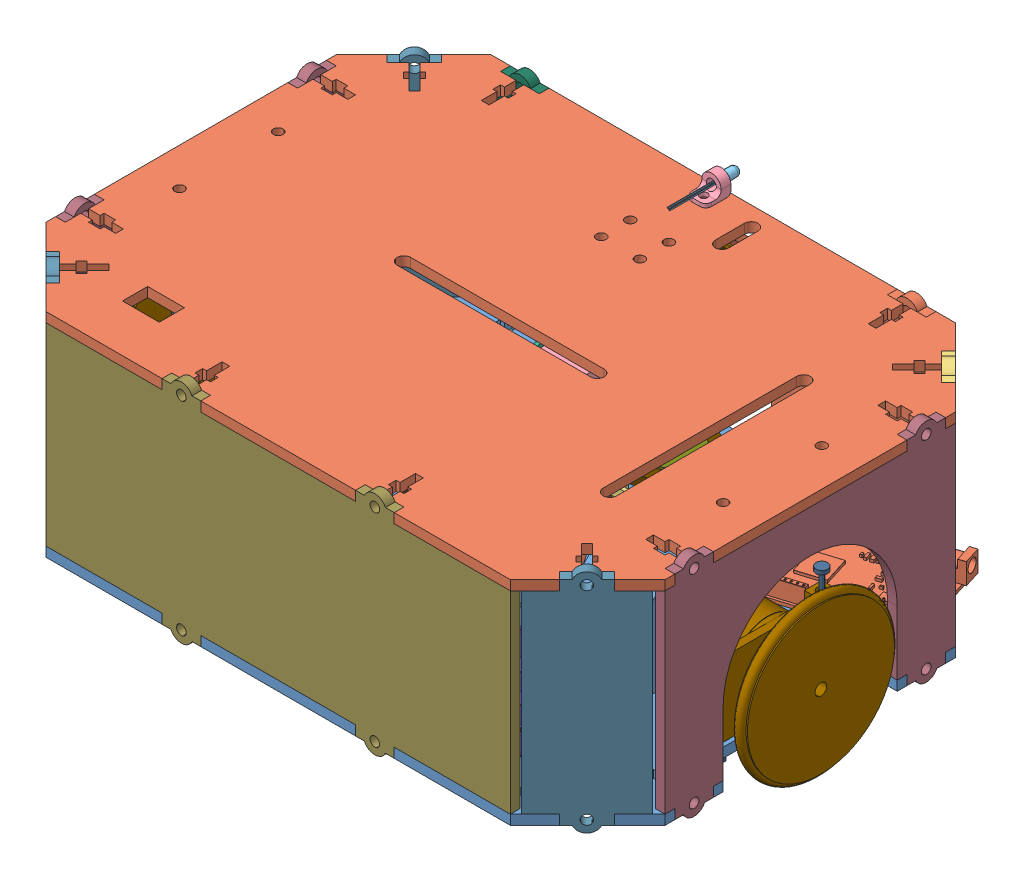
SolidWorks assembly Prototype-Conception, configuration Default. Lengths in mm.
Overall size (331.14 134.32 253.47).
132 component instances, 59 part files, 49 mates.
Components (placement in the parent):
- prototype1_base1-1: prototype1_base1 [Default] at (144.9851 187.411 243.3033) size (320 5 230)
- ArduinoMega-2: ArduinoMega [Default] at (236.0783 194.062 168.5879) x (0.955339 0 -0.295511) z (0 -1 0) size (107.95 53.42 12.95)
- L298N Stepper drive-1: L298N Stepper drive [Default] at (148.4735 192.411 198.6187) x (0 0 1) z (-1 0 0) size (25 6 25)
- servo+support-1: servo+support [Default] at (76.7363 185.3539 129.6171) size (30.85 17.44 63.47)
  - Servo SG90-1: Servo SG90 [Predeterminado] at (16.5878 18.2571 21.1863) x (0 0 -1) z (0 1 0) size (32.1 30.85 12.4)
  - support servo-1: support servo [Default] at (18.3998 7.0571 21.1863) size (20 17 35)
  - MG995.step-1: MG995.step [Default] at (-1.5122 18.2571 16.1363) x (0 0.99966 -0.026078) z (1 0 0) size (11.5 38 5)
  - ebra-1: ebra [Default] at (-1.6485 18.0008 3.8517) x (0.943956 0.329772 -0.014044) z (-0.330071 0.943101 -0.040165) size (0.5 28.65 0.5)
- battery_holder.step-1: battery_holder.step [Default] at (221.2091 192.411 308.7692) x (-0.012882 0 0.999917) z (-0.999917 0 -0.012882) size (48.1 20.2 69.05)
- encodeur-support-1: encodeur-support [Défaut] at (-4.8153 224.4568 275.8648) x (0 0 -1) z (0 1 0) size (81 60.27 81)
- tige-1: tige [Default] at (4.4851 181.5741 217.8033) x (0.335505 0 -0.942038) z (0.942038 0 0.335505) size (6 62 6)
- tige-2: tige [Default] at (4.4851 182.0721 268.8033) x (0.721195 0 -0.692732) z (0.692732 0 0.721195) size (6 62 6)
- encodeur-support-2: encodeur-support [Défaut] at (294.7855 202.7294 275.8648) x (0 0 -1) z (0 -1 0) size (81 60.27 81)
- tige-3: tige [Default] at (285.4851 182.0721 268.8033) x (-0.721195 0 -0.692732) z (0.692732 0 -0.721195) size (6 62 6)
- tige-4: tige [Default] at (285.4851 181.5741 217.8033) x (-0.335505 0 -0.942038) z (0.942038 0 -0.335505) size (6 62 6)
- JGB37-520-1: JGB37-520 [Default] at (205.9851 219.6351 243.2582) x (0 0.001856 -0.999998) z (1 0 0) size (39.09 46.73 78.38)
  - GEARED BODY, MOTOR, JGB37-520-1-1: GEARED BODY, MOTOR, JGB37-520-1 [Default] at origin size (37 37 29)
  - DC MOTOR, JGB37-520-1-1: DC MOTOR, JGB37-520-1 [Default] at (0 0 -29) x (-1 0 0) z (0 0 1) size (33 33 19.5)
  - MOTOR SHAFT, JGB37-520-1-1: MOTOR SHAFT, JGB37-520-1 [Default] at (0 7 0) x (-0.942506 0.334191 0) z (0 0 1) size (6 6 21.5)
  - SHAFT COUPLER, JGB37-520-1-1: SHAFT COUPLER, JGB37-520-1 [Default] at (0 7 0) x (0.631787 0.775142 0) z (0 0 1) size (12 12 6)
  - COUPLING BRACKET, GEARED BODY TO DC MOTOR, JGB37-520-1-1: COUPLING BRACKET, GEARED BODY TO DC MOTOR, JGB37-520-1 [Default] at (0 0 -25) size (34 34 4)
  - PLASTIC COVER, DC MOTOR, JGB37-520-1-1: PLASTIC COVER, DC MOTOR, JGB37-520-1 [Default] at (0 0 -48.5) size (33 33 8.5)
  - CONNECTION, DC MOTOR, JGB37-520-1-1: CONNECTION, DC MOTOR, JGB37-520-1 [Default] at (0 -12.8 -50.25) x (1 0 0) z (0 0 -1) size (3 3.62 10.88)
  - CONNECTION, DC MOTOR, JGB37-520-1-2: CONNECTION, DC MOTOR, JGB37-520-1 [Default] at (0 12.8 -50.25) x (-1 0 0) z (0 0 -1) size (3 3.62 10.88)
  - pan cross head_am(B18.6.7M - M2 x 0.4 x 25 Type I Cross Recessed PHMS --25N)-1: pan cross head_am(B18.6.7M - M2 x 0.4 x 25 Type I Cross Recessed PHMS --25N) [Default] at (13.4234 7.75 0) x (0 0 -1) z (0.597515 0.801858 0) size (26.58 4 4)
  - pan cross head_am(B18.6.7M - M2 x 0.4 x 25 Type I Cross Recessed PHMS --25N)-2: pan cross head_am(B18.6.7M - M2 x 0.4 x 25 Type I Cross Recessed PHMS --25N) [Default] at (-13.4234 7.75 0) x (0 0 -1) z (-0.993187 0.116535 0) size (26.58 4 4)
  - pan cross head_am(B18.6.7M - M2 x 0.4 x 25 Type I Cross Recessed PHMS --25N)-3: pan cross head_am(B18.6.7M - M2 x 0.4 x 25 Type I Cross Recessed PHMS --25N) [Default] at (0 -15.5 0) x (0 0 -1) z (0.395671 -0.918392 0) size (26.58 4 4)
  - support motor-1: support motor [Default] at (19.4043 -27.2602 2) x (-0.999998 0.001856 0) z (0 0 -1) size (39 46.66 42)
- JGB37-520-2: JGB37-520 [Default] at (83.9851 219.6349 243.3629) x (0 -0.001856 0.999998) z (-1 0 0) size (39.09 46.73 78.38)
  - GEARED BODY, MOTOR, JGB37-520-1-1: GEARED BODY, MOTOR, JGB37-520-1 [Default] at origin size (37 37 29)
  - DC MOTOR, JGB37-520-1-1: DC MOTOR, JGB37-520-1 [Default] at (0 0 -29) x (-1 0 0) z (0 0 1) size (33 33 19.5)
  - MOTOR SHAFT, JGB37-520-1-1: MOTOR SHAFT, JGB37-520-1 [Default] at (0 7 0) x (-0.942506 0.334191 0) z (0 0 1) size (6 6 21.5)
  - SHAFT COUPLER, JGB37-520-1-1: SHAFT COUPLER, JGB37-520-1 [Default] at (0 7 0) x (0.631787 0.775142 0) z (0 0 1) size (12 12 6)
  - COUPLING BRACKET, GEARED BODY TO DC MOTOR, JGB37-520-1-1: COUPLING BRACKET, GEARED BODY TO DC MOTOR, JGB37-520-1 [Default] at (0 0 -25) size (34 34 4)
  - PLASTIC COVER, DC MOTOR, JGB37-520-1-1: PLASTIC COVER, DC MOTOR, JGB37-520-1 [Default] at (0 0 -48.5) size (33 33 8.5)
  - CONNECTION, DC MOTOR, JGB37-520-1-1: CONNECTION, DC MOTOR, JGB37-520-1 [Default] at (0 -12.8 -50.25) x (1 0 0) z (0 0 -1) size (3 3.62 10.88)
  - CONNECTION, DC MOTOR, JGB37-520-1-2: CONNECTION, DC MOTOR, JGB37-520-1 [Default] at (0 12.8 -50.25) x (-1 0 0) z (0 0 -1) size (3 3.62 10.88)
  - pan cross head_am(B18.6.7M - M2 x 0.4 x 25 Type I Cross Recessed PHMS --25N)-1: pan cross head_am(B18.6.7M - M2 x 0.4 x 25 Type I Cross Recessed PHMS --25N) [Default] at (13.4234 7.75 0) x (0 0 -1) z (0.597515 0.801858 0) size (26.58 4 4)
  - pan cross head_am(B18.6.7M - M2 x 0.4 x 25 Type I Cross Recessed PHMS --25N)-2: pan cross head_am(B18.6.7M - M2 x 0.4 x 25 Type I Cross Recessed PHMS --25N) [Default] at (-13.4234 7.75 0) x (0 0 -1) z (-0.993187 0.116535 0) size (26.58 4 4)
  - pan cross head_am(B18.6.7M - M2 x 0.4 x 25 Type I Cross Recessed PHMS --25N)-3: pan cross head_am(B18.6.7M - M2 x 0.4 x 25 Type I Cross Recessed PHMS --25N) [Default] at (0 -15.5 0) x (0 0 -1) z (0.395671 -0.918392 0) size (26.58 4 4)
  - support motor-1: support motor [Default] at (19.4043 -27.2602 2) x (-0.999998 0.001856 0) z (0 0 -1) size (39 46.66 42)
- battery_holder.step-2: battery_holder.step [Default] at (56.2097 192.411 316.6119) x (0 0 1) z (-1 0 0) size (48.1 20.2 69.05)
- base2-1: base2 [Default] at (20.8896 140.0145 -8.0898) size (320 60 230.9)
  - prototype1_base2-1: prototype1_base2 [Default] at (124.0955 152.3965 251.3932) size (320 5 230)
  - ESP3-CAM v44-1: ESP3-CAM v44 [Default] at (110.5829 141.6845 144.5621) x (0 -1 0) z (1 0 0) size (55 63.9 40.58)
    - ESP3-CAM v4.step-1: ESP3-CAM v4.step [Default] at origin size (40.5 18.08 27)
      - ESp32-WROOM-32U v3.step-1: ESp32-WROOM-32U v3.step [Default] at (15.3712 -0.1455 22.8712) x (0 0 -1) z (-1 0 0) size (18.07 3.43 19.24)
        - u.step-1: u.step [Default] at (15.6609 1 -15.1484) x (0 0 -1) z (1 0 0) size (3.1 1.25 3)
        - ESp32-WROOM-32U v3-0.step-1: ESp32-WROOM-32U v3-0.step [Default] at origin size (18.07 3.43 19.24)
      - sop127p-6mm-8 v2.step-1: sop127p-6mm-8 v2.step [Default] at (4 0 7) x (0 0 1) z (0 -1 0) size (4.9 5.9 1.65)
        - icbody.step-1: icbody.step [Default] at origin size (4.9 3.9 1.45)
        - Component5.step-1: Component5.step [Default] at origin size (0.4 1 1.05)
        - Component5.step-2: Component5.step [Default] at (1.27 0 0) size (0.4 1 1.05)
        - Component5.step-3: Component5.step [Default] at (-1.27 0 0) size (0.4 1 1.05)
        - Component5.step-4: Component5.step [Default] at (-2.54 0 0) size (0.4 1 1.05)
        - Component5(Mirror).step-1: Component5(Mirror).step [Default] at (-1.27 0 0) x (1 0 0) z (0 0 -1) size (0.4 1 1.05)
        - Component5(Mirror).step-2: Component5(Mirror).step [Default] at (1.27 0 0) x (1 0 0) z (0 0 -1) size (0.4 1 1.05)
        - Component5(Mirror).step-3: Component5(Mirror).step [Default] x (1 0 0) z (0 0 -1) size (0.4 1 1.05)
        - Component5(Mirror).step-4: Component5(Mirror).step [Default] at (-2.54 0 0) x (1 0 0) z (0 0 -1) size (0.4 1 1.05)
      - SMD LED 0603.step-1: SMD LED 0603.step [Default] at (12 0 18) x (0 0 1) z (0 -1 0) size (1.6 0.8 0.6)
        - Fusion.step-1: Fusion.step [Default] at origin size (1.6 0.8 0.5)
        - Fillet.step-1: Fillet.step [Default] at origin size (1.2 0.8 0.3)
      - MicroSD Slot.step-1: MicroSD Slot.step [Default] at (26.7 3 17.2) x (1 0 0) z (0 1 0) size (15 16 2)
        - sdreader.step-1: sdreader.step [Default] at (-11.2744 2.632 -3.2) size (15 16 2)
      - camera for ESP32.step-1: camera for ESP32.step [Default] at (24.1466 3.3198 13.5126) x (0 0 -1) z (0 1 0) size (12.5 21.5 6.03)
        - User Library-ov9655_ov9655_flex_pcb.step-1: User Library-ov9655_ov9655_flex_pcb.step [Default] at origin size (12.5 21.5 0.12)
        - User Library-ov9655_ov9655_flex_reinf.step-1: User Library-ov9655_ov9655_flex_reinf.step [Default] at origin size (12.5 4.5 0.25)
        - User Library-ov9655_ov9655_back_panel.step-1: User Library-ov9655_ov9655_back_panel.step [Default] at origin size (8.5 8.5 0.25)
        - User Library-ov9655_ov9655_body.step-1: User Library-ov9655_ov9655_body.step [Default] at origin size (8.5 8.5 6.03)
        - User Library-ov9655_ov9655_lens.step-1: User Library-ov9655_ov9655_lens.step [Default] at origin size (2 2 1.43)
      - Pin Header 4 x 1 TH 2.54mm Pitch.step-1: Pin Header 4 x 1 TH 2.54mm Pitch.step [Default] at (4.72 -2.6622 2.2022) x (0 0 1) z (0 1 0) size (2.54 10.16 11.43)
      - Pin Header 4 x 1 TH 2.54mm Pitch.step-2: Pin Header 4 x 1 TH 2.54mm Pitch.step [Default] at (14.883 -2.6622 2.2022) x (0 0 1) z (0 1 0) size (2.54 10.16 11.43)
      - Pin Header 4 x 1 TH 2.54mm Pitch.step-3: Pin Header 4 x 1 TH 2.54mm Pitch.step [Default] at (14.89 -2.6622 25.2022) x (0 0 1) z (0 1 0) size (2.54 10.16 11.43)
      - Pin Header 4 x 1 TH 2.54mm Pitch.step-4: Pin Header 4 x 1 TH 2.54mm Pitch.step [Default] at (4.71 -2.6622 25.2022) x (0 0 1) z (0 1 0) size (2.54 10.16 11.43)
      - capacitor-CAPM-TANTB-YL.step-1: capacitor-CAPM-TANTB-YL.step [Default] at (11 0.105 22.105) x (1 0 0) z (0 -1 0) size (3.7 3 2.1)
      - switch-3x4x2mm - 2 Pad.step-1: switch-3x4x2mm - 2 Pad.step [Default] at (4 0.685 21.7704) x (1 0 0) z (0 -1 0) size (5 3 1.93)
      - nano - reg.step-1: nano - reg.step [Default] at (4.45 -0.0047 14.7657) x (0 0 -1) z (-1 0 0) size (6.5 1.69 8.3)
      - resistor-NTC-0402-T0.6.step-1: resistor-NTC-0402-T0.6.step [Default] at (12.2 0 15.8) x (0 0 -1) z (1 0 0) size (1.1 0.55 0.6)
      - resistor-NTC-0402-T0.6.step-2: resistor-NTC-0402-T0.6.step [Default] at (10.2 0 12.3) x (0 0 -1) z (1 0 0) size (1.1 0.55 0.6)
      - resistor-NTC-0402-T0.6.step-3: resistor-NTC-0402-T0.6.step [Default] at (11.2 0 5.9714) x (0 0 -1) z (1 0 0) size (1.1 0.55 0.6)
      - resistor-NTC-0805-T1.3.step-1: resistor-NTC-0805-T1.3.step [Default] at (10.35 0 14.65) x (0 0 -1) z (1 0 0) size (2.2 1.4 1.3)
      - resistor-NTC-0402-T0.6.step-4: resistor-NTC-0402-T0.6.step [Default] at (4.5 0 10.6) x (-1 0 0) z (0 0 -1) size (1.1 0.55 0.6)
      - resistor-NTC-0402-T0.6.step-5: resistor-NTC-0402-T0.6.step [Default] at (25.5 0 24.5) size (1.1 0.55 0.6)
      - resistor-NTC-0402-T0.6.step-6: resistor-NTC-0402-T0.6.step [Default] at (28.5 0 24.5) size (1.1 0.55 0.6)
      - resistor-NTC-0402-T0.6.step-7: resistor-NTC-0402-T0.6.step [Default] at (32.5 0 24.5) size (1.1 0.55 0.6)
      - smd-transistor-SOT23-3.step-1: smd-transistor-SOT23-3.step [Default] at (27 1.058 2.442) x (1 0 0) z (0 1 0) size (2.84 3.01 1.19)
      - smd-transistor-SOT23-3.step-2: smd-transistor-SOT23-3.step [Default] at (27 1.058 23.942) x (1 0 0) z (0 1 0) size (2.84 3.01 1.19)
      - resistor-NTC-0402-T0.6.step-8: resistor-NTC-0402-T0.6.step [Default] at (29.3 1 24.3) x (0 0 1) z (-1 0 0) size (1.1 0.55 0.6)
      - resistor-NTC-0402-T0.6.step-9: resistor-NTC-0402-T0.6.step [Default] at (30.3 1 24.3) x (0 0 1) z (-1 0 0) size (1.1 0.55 0.6)
      - resistor-NTC-0402-T0.6.step-10: resistor-NTC-0402-T0.6.step [Default] at (31 1 17) size (1.1 0.55 0.6)
      - LED SMD 5050 White.step-1: LED SMD 5050 White.step [Default] at (30 1.2963 2.1003) x (1 0 0) z (0 1 0) size (5.4 5 1.62)
      - resistor-NTC-0402-T0.6.step-11: resistor-NTC-0402-T0.6.step [Default] at (20.7 1 4.3) x (0 0 -1) z (1 0 0) size (1.1 0.55 0.6)
      - resistor-NTC-0402-T0.6.step-12: resistor-NTC-0402-T0.6.step [Default] at (19.7 1 4.3) x (0 0 -1) z (1 0 0) size (1.1 0.55 0.6)
      - resistor-NTC-0402-T0.6.step-13: resistor-NTC-0402-T0.6.step [Default] at (18.7 1 4.3) x (0 0 -1) z (1 0 0) size (1.1 0.55 0.6)
      - resistor-NTC-0402-T0.6.step-14: resistor-NTC-0402-T0.6.step [Default] at (17.7 1 4.3) x (0 0 -1) z (1 0 0) size (1.1 0.55 0.6)
      - resistor-NTC-0402-T0.6.step-15: resistor-NTC-0402-T0.6.step [Default] at (21 1 5.2) size (1.1 0.55 0.6)
      - resistor-NTC-0402-T0.6.step-16: resistor-NTC-0402-T0.6.step [Default] at (18 1 6.2) size (1.1 0.55 0.6)
      - resistor-NTC-0402-T0.6.step-17: resistor-NTC-0402-T0.6.step [Default] at (18 1 7.2) size (1.1 0.55 0.6)
      - capacitor-CAPC-0603-T0.9-BN.step-1: capacitor-CAPC-0603-T0.9-BN.step [Default] at (21 1 7) size (1.7 0.9 0.9)
      - resistor-NTC-0402-T0.6.step-18: resistor-NTC-0402-T0.6.step [Default] at (21 1 6) size (1.1 0.55 0.6)
      - capacitor-CAPC-0603-T0.9-BN.step-2: capacitor-CAPC-0603-T0.9-BN.step [Default] at (22 1 21) size (1.7 0.9 0.9)
      - smd-transistor-SOT23-3.step-3: smd-transistor-SOT23-3.step [Default] at (21.5739 1.058 19.0158) x (0 0 -1) z (0 1 0) size (2.84 3.01 1.19)
      - connector smd usl00-20l_p0-4_l12-6_w2-75.step-1: connector smd usl00-20l_p0-4_l12-6_w2-75.step [Default] at (26.791 1 14.009) x (0 0 -1) z (1 0 0) size (12.6 1 3.1)
      - resistor-NTC-0402-T0.6.step-19: resistor-NTC-0402-T0.6.step [Default] at (18 1 14.2) size (1.1 0.55 0.6)
      - resistor-NTC-0402-T0.6.step-20: resistor-NTC-0402-T0.6.step [Default] at (18 1 13.2) size (1.1 0.55 0.6)
      - smd-transistor-SOT23-3.step-4: smd-transistor-SOT23-3.step [Default] at (21.5739 1.058 10.0158) x (0 0 -1) z (0 1 0) size (2.84 3.01 1.19)
      - Micro SD-Card.step-1: Micro SD-Card.step [Default] at (7 2.64 12.5) size (15 1.01 11)
      - ESP3-CAM.step-1: ESP3-CAM.step [Default] at origin size (40 1 27)
    - ESP32-CAM-MB.step-2: ESP32-CAM-MB.step [Default] at (20 -12.6622 13.5) x (0 0 -1) z (1 0 0) size (29 11.5 40.1)
    - camsupport2-1: camsupport2 [Default] at (21.788 -19.8311 13.5126) size (55 63 40.58)
- backwall-1: backwall [Default] at (144.9851 242.411 353.3033) size (240 117 5)
- encoderwall-1: encoderwall [Default] at (-15.0149 242.411 243.3033) x (0 0 -1) z (1 0 0) size (150 117 5)
- encoderwall-2: encoderwall [Default] at (299.9851 242.411 243.3033) x (0 0 -1) z (1 0 0) size (150 117 5)
- coinwall-1: coinwall [Default] at (5.1861 242.411 338.5044) x (-0.707107 0 -0.707107) z (0.707107 0 -0.707107) size (48 117 5)
- coinwall-3: coinwall [Default] at (8.7216 242.411 151.6379) x (-0.707107 0 0.707107) z (-0.707107 0 -0.707107) size (48 117 5)
- frontwall-1: frontwall [Default] at (44.9851 242.411 128.3033) size (40 117 5)
- roue libre-4: roue libre [Défaut] at (146.6321 249.2451 156.3537) x (-0.999947 0 0.010315) z (0 -1 0) size (63.51 43.75 22.8)
  - roue libre part 2-1: roue libre part 2 [Défaut] at (-21.9143 1.2898 50.7632) size (51.26 32 1)
  - roue libre part 1-1: roue libre part 1 [Défaut] at (1.9577 -1.6099 47.7186) x (0.915865 -0.401487 0) z (0 0 -1) size (29 29 21.8)
  - scroller support-1: scroller support [Default] at (1.7188 -1.9676 51.7865) x (-0.999928 -0.011969 0) z (-0.011969 0.999928 0) size (63 5 43)
- roue-1: roue [Default] at (44.0134 208.9613 242.8807) x (0 -0.093585 -0.995611) z (1 0 0) size (65 65 35)
- roue-2: roue [Default] at (210.9568 208.9613 242.8807) x (0 -0.093585 -0.995611) z (1 0 0) size (65 65 35)
- roue libre-5: roue libre [Défaut] at (146.6727 249.2451 326.318) x (-0.999947 0 -0.010315) z (0 -1 0) size (63.51 43.75 22.8)
  - roue libre part 2-1: roue libre part 2 [Défaut] at (-21.9143 1.2898 50.7632) size (51.26 32 1)
  - roue libre part 1-1: roue libre part 1 [Défaut] at (1.9577 -1.6099 47.7186) x (0.915865 -0.401487 0) z (0 0 -1) size (29 29 21.8)
  - scroller support-1: scroller support [Default] at (1.7188 -1.9676 51.7865) x (-0.999928 -0.011969 0) z (-0.011969 0.999928 0) size (63 5 43)
- frontwallleft-1: frontwallleft [Default] at (219.9851 242.411 133.3033) x (-1 0 0) z (0 0 -1) size (90 117 5)
- coinwallarduino-1: coinwallarduino [Default] at (284.7841 242.411 148.1023) x (0.707107 0 0.707107) z (-0.707107 0 0.707107) size (48 88.5 5)
- coinwall-5: coinwall [Default] at (281.2485 242.411 334.9688) x (0.707107 0 -0.707107) z (0.707107 0 0.707107) size (48 117 5)
- led1-1: led1 [Default] at (141.8283 292.4605 120.5811) size (10 10 36.5)
  - led support-1: led support [Default] at (3.1568 9.9504 8.7223) size (10 10 13)
  - LED 5mm.step-1: LED 5mm.step [Default] at (3.1568 9.9504 8.7223) x (0.923728 0.383049 0) z (-0.383049 0.923728 0) size (5.2 36.5 5.5)
Mates (geometry in assembly coordinates):
- Coincident16: coincident anti-aligned: plane of prototype1_base1-1 through (144.9851 192.411 243.3033) normal (0 1 0); plane of ArduinoMega-2 through (276.717 192.411 128.0607) normal (0 -1 0)
- Coincident17: coincident anti-aligned: plane of prototype1_base1-1 through (144.9851 192.411 243.3033) normal (0 1 0); plane of L298N Stepper drive-1 through (148.4735 192.411 198.6187) normal (0 -1 0)
- Distance1: distance = 5 mm aligned: plane of servo+support-1/support servo-1 through (105.1361 197.411 133.3033) normal (0 0 -1); plane of prototype1_base1-1 through (304.9851 192.411 128.3033) normal (0 0 -1)
- Coincident20: coincident anti-aligned: plane of prototype1_base1-1 through (144.9851 192.411 243.3033) normal (0 1 0); plane of servo+support-1/support servo-1 through (95.1361 192.411 150.8033) normal (0 -1 0)
- Coincident21: coincident anti-aligned: plane of prototype1_base1-1 through (144.9851 192.411 243.3033) normal (0 1 0); plane of battery_holder.step-1 through (221.2091 192.411 308.7692) normal (0 -1 0)
- Width1: width anti-aligned: plane of encodeur-support-1 through (-0.0149 232.5931 273.3033) normal (0 0 1); plane of prototype1_base1-1 through (-0.0149 232.5931 213.3033) normal (0 0 -1); plane of encodeur-support-1 through (-15.0149 187.411 288.3033) normal (0 0 -1); plane of prototype1_base1-1 through (-15.0149 187.411 198.3033) normal (0 0 1)
- Coincident24: coincident aligned: plane of prototype1_base1-1 through (-0.0149 187.411 198.3033) normal (-1 0 0); plane of encodeur-support-1 through (-0.0149 232.5931 273.3033) normal (-1 0 0)
- Concentric2: concentric aligned: cylinder of encodeur-support-1 through (4.4851 232.5931 217.8033) axis (0 -1 0) radius 2.5; cylinder of tige-1 through (4.4851 241.5741 217.8033) axis (0 -1 0) radius 1.1
- Concentric3: concentric aligned: cylinder of encodeur-support-1 through (4.4851 232.5931 268.8033) axis (0 -1 0) radius 2.5; cylinder of tige-2 through (4.4851 242.0721 268.8033) axis (0 -1 0) radius 1.1
- Coincident34: coincident anti-aligned: plane of prototype1_base1-1 through (144.9851 192.411 243.3033) normal (0 1 0); plane of JGB37-520-1/support motor-1 through (205.9851 192.411 223.8033) normal (0 -1 0)
- Width3: width anti-aligned: plane of JGB37-520-1/support motor-1 through (205.9851 192.411 223.8033) normal (0 0 -1); plane of JGB37-520-1/support motor-1 through (205.9851 192.411 262.8033) normal (0 0 1); plane of prototype1_base1-1 through (247.9851 187.411 205.8033) normal (0 0 1); plane of prototype1_base1-1 through (247.9851 187.411 280.8033) normal (0 0 -1)
- Coincident35: coincident aligned: plane of prototype1_base1-1 through (207.9851 187.411 205.8033) normal (1 0 0); plane of JGB37-520-1/support motor-1 through (207.9851 219.5706 243.3026) normal (1 0 0)
- Coincident37: coincident anti-aligned: plane of prototype1_base1-1 through (144.9851 192.411 243.3033) normal (0 1 0); plane of battery_holder.step-2 through (56.2097 192.411 316.6119) normal (0 -1 0)
- Width6: width aligned: plane of base2-1/prototype1_base2-1 through (-15.0149 297.411 358.3033) normal (-1 0 0); plane of prototype1_base1-1 through (304.9851 297.411 358.3033) normal (1 0 0); plane of base2-1/prototype1_base2-1 through (-15.0149 192.411 358.3033) normal (-1 0 0); plane of prototype1_base1-1 through (304.9851 192.411 358.3033) normal (1 0 0)
- Width7: width aligned: plane of base2-1/prototype1_base2-1 through (304.9851 297.411 358.3033) normal (0 0 1); plane of prototype1_base1-1 through (304.9851 297.411 128.3033) normal (0 0 -1); plane of base2-1/prototype1_base2-1 through (304.9851 192.411 358.3033) normal (0 0 1); plane of prototype1_base1-1 through (304.9851 192.411 128.3033) normal (0 0 -1)
- Distance3: distance = 100 mm anti-aligned: plane of prototype1_base1-1 through (144.9851 192.411 243.3033) normal (0 1 0); plane of base2-1/prototype1_base2-1 through (144.9851 292.411 243.3033) normal (0 -1 0)
- Coincident40: coincident anti-aligned: plane of base2-1/prototype1_base2-1 through (104.9851 287.411 353.3033) normal (0 0 1); plane of backwall-1 through (144.9851 242.411 353.3033) normal (0 0 -1)
- Coincident41: coincident anti-aligned: plane of base2-1/prototype1_base2-1 through (104.9851 287.411 358.3033) normal (-1 0 0); plane of backwall-1 through (104.9851 297.411 353.3033) normal (1 0 0)
- Coincident42: coincident aligned: plane of base2-1/prototype1_base2-1 through (144.9851 297.411 243.3033) normal (0 1 0); plane of backwall-1 through (144.9851 297.411 353.3033) normal (0 1 0)
- Coincident43: coincident anti-aligned: plane of base2-1/prototype1_base2-1 through (-10.0149 287.411 243.3033) normal (-1 0 0); plane of encoderwall-1 through (-10.0149 242.411 243.3033) normal (1 0 0)
- Coincident44: coincident anti-aligned: plane of base2-1/prototype1_base2-1 through (144.9851 287.411 193.3033) normal (0 0 -1); plane of encoderwall-1 through (-15.0149 297.411 193.3033) normal (0 0 1)
- Coincident45: coincident anti-aligned: plane of base2-1/prototype1_base2-1 through (144.9851 292.411 243.3033) normal (0 -1 0); plane of encoderwall-1 through (-10.0149 292.411 168.3033) normal (0 1 0)
- Coincident46: coincident anti-aligned: plane of base2-1/prototype1_base2-1 through (299.9851 287.411 243.3033) normal (1 0 0); plane of encoderwall-2 through (299.9851 242.411 243.3033) normal (-1 0 0)
- Coincident47: coincident anti-aligned: plane of base2-1/prototype1_base2-1 through (144.9851 292.411 243.3033) normal (0 -1 0); plane of encoderwall-2 through (304.9851 292.411 168.3033) normal (0 1 0)
- Coincident48: coincident anti-aligned: plane of base2-1/prototype1_base2-1 through (144.9851 287.411 313.3033) normal (0 0 -1); plane of encoderwall-2 through (299.9851 297.411 313.3033) normal (0 0 1)
- Coincident49: coincident anti-aligned: plane of base2-1/prototype1_base2-1 through (31.0206 287.411 357.2678) normal (-0.707107 0 0.707107); plane of coinwall-1 through (8.7216 242.411 334.9688) normal (0.707107 0 -0.707107)
- Coincident50: coincident anti-aligned: plane of base2-1/prototype1_base2-1 through (129.7572 287.411 228.0754) normal (-0.707107 0 -0.707107); plane of coinwall-1 through (15.7927 297.411 342.0399) normal (0.707107 0 0.707107)
- Coincident51: coincident anti-aligned: plane of base2-1/prototype1_base2-1 through (144.9851 292.411 243.3033) normal (0 -1 0); plane of coinwall-1 through (-8.2489 292.411 317.9983) normal (0 1 0)
- Coincident56: coincident anti-aligned: plane of base2-1/prototype1_base2-1 through (129.7572 287.411 258.5313) normal (-0.707107 0 0.707107); plane of coinwall-3 through (12.2572 297.411 141.0313) normal (0.707107 0 -0.707107)
- Coincident59: coincident anti-aligned: plane of base2-1/prototype1_base2-1 through (129.7572 287.411 258.5313) normal (-0.707107 0 0.707107); plane of coinwall-3 through (12.2572 297.411 141.0313) normal (0.707107 0 -0.707107)
- Coincident60: coincident anti-aligned: plane of base2-1/prototype1_base2-1 through (115.615 287.411 272.6734) normal (0.707107 0 -0.707107); plane of coinwall-3 through (-1.885 297.411 155.1734) normal (-0.707107 0 0.707107)
- Coincident61: coincident anti-aligned: plane of base2-1/prototype1_base2-1 through (31.0206 287.411 129.3389) normal (-0.707107 0 -0.707107); plane of coinwall-3 through (8.7216 242.411 151.6379) normal (0.707107 0 0.707107)
- Coincident62: coincident anti-aligned: plane of base2-1/prototype1_base2-1 through (144.9851 292.411 243.3033) normal (0 -1 0); plane of coinwall-3 through (-11.7845 292.411 165.0729) normal (0 1 0)
- Coincident66: coincident anti-aligned: plane of base2-1/prototype1_base2-1 through (54.9851 287.411 243.3033) normal (-1 0 0); plane of frontwall-1 through (54.9851 297.411 133.3033) normal (1 0 0)
- Coincident67: coincident anti-aligned: plane of base2-1/prototype1_base2-1 through (144.9851 287.411 133.3033) normal (0 0 -1); plane of frontwall-1 through (44.9851 242.411 133.3033) normal (0 0 1)
- Coincident68: coincident anti-aligned: plane of base2-1/prototype1_base2-1 through (144.9851 292.411 243.3033) normal (0 -1 0); plane of frontwall-1 through (64.9851 292.411 133.3033) normal (0 1 0)
- Concentric23: concentric aligned: cylinder of prototype1_base1-1 through (123.4337 182.411 158.3033) axis (0 1 0) radius 3.5; cylinder of roue libre-4/roue libre part 2-1 through (123.4337 197.482 158.3033) axis (0 1 0) radius 2.5
- Coincident69: coincident aligned: plane of base2-1/prototype1_base2-1 through (304.9851 297.411 128.3033) normal (0 0 -1); plane of frontwallleft-1 through (219.9851 242.411 128.3033) normal (0 0 -1)
- Coincident70: coincident anti-aligned: plane of base2-1/prototype1_base2-1 through (144.9851 292.411 243.3033) normal (0 -1 0); plane of frontwallleft-1 through (174.9851 292.411 128.3033) normal (0 1 0)
- Coincident71: coincident anti-aligned: plane of base2-1/prototype1_base2-1 through (234.9851 287.411 243.3033) normal (1 0 0); plane of frontwallleft-1 through (234.9851 297.411 128.3033) normal (-1 0 0)
- Coincident72: coincident anti-aligned: plane of base2-1/prototype1_base2-1 through (258.9496 287.411 129.3389) normal (0.707107 0 -0.707107); plane of coinwallarduino-1 through (281.2485 242.411 151.6379) normal (-0.707107 0 0.707107)
- Coincident73: coincident anti-aligned: plane of base2-1/prototype1_base2-1 through (174.3551 287.411 272.6734) normal (-0.707107 0 -0.707107); plane of coinwallarduino-1 through (288.3196 297.411 158.7089) normal (0.707107 0 0.707107)
- Coincident74: coincident anti-aligned: plane of base2-1/prototype1_base2-1 through (144.9851 292.411 243.3033) normal (0 -1 0); plane of coinwallarduino-1 through (298.2191 292.411 168.6084) normal (0 1 0)
- Coincident75: coincident anti-aligned: plane of base2-1/prototype1_base2-1 through (258.9496 287.411 357.2678) normal (0.707107 0 0.707107); plane of coinwall-5 through (281.2485 242.411 334.9688) normal (-0.707107 0 -0.707107)
- Coincident76: coincident anti-aligned: plane of base2-1/prototype1_base2-1 through (144.9851 292.411 243.3033) normal (0 -1 0); plane of coinwall-5 through (301.7546 292.411 321.5338) normal (0 1 0)
- Coincident77: coincident anti-aligned: plane of base2-1/prototype1_base2-1 through (174.3551 287.411 213.9333) normal (-0.707107 0 0.707107); plane of coinwall-5 through (291.8551 297.411 331.4333) normal (0.707107 0 -0.707107)
- Concentric24: concentric aligned: cylinder of base2-1/prototype1_base2-1 through (144.9851 289.411 138.3033) axis (0 1 0) radius 2; cylinder of led1-1/led support-1 through (144.9851 291.411 138.3033) axis (0 1 0) radius 2
- Coincident80: coincident anti-aligned: plane of base2-1/prototype1_base2-1 through (144.9851 297.411 243.3033) normal (0 1 0); plane of led1-1/led support-1 through (149.9851 297.411 134.3033) normal (0 -1 0)
- Parallel1: parallel aligned: plane of base2-1/prototype1_base2-1 through (304.9851 297.411 128.3033) normal (0 0 -1); plane of led1-1/led support-1 through (144.9851 302.411 129.3033) normal (0 0 -1)
